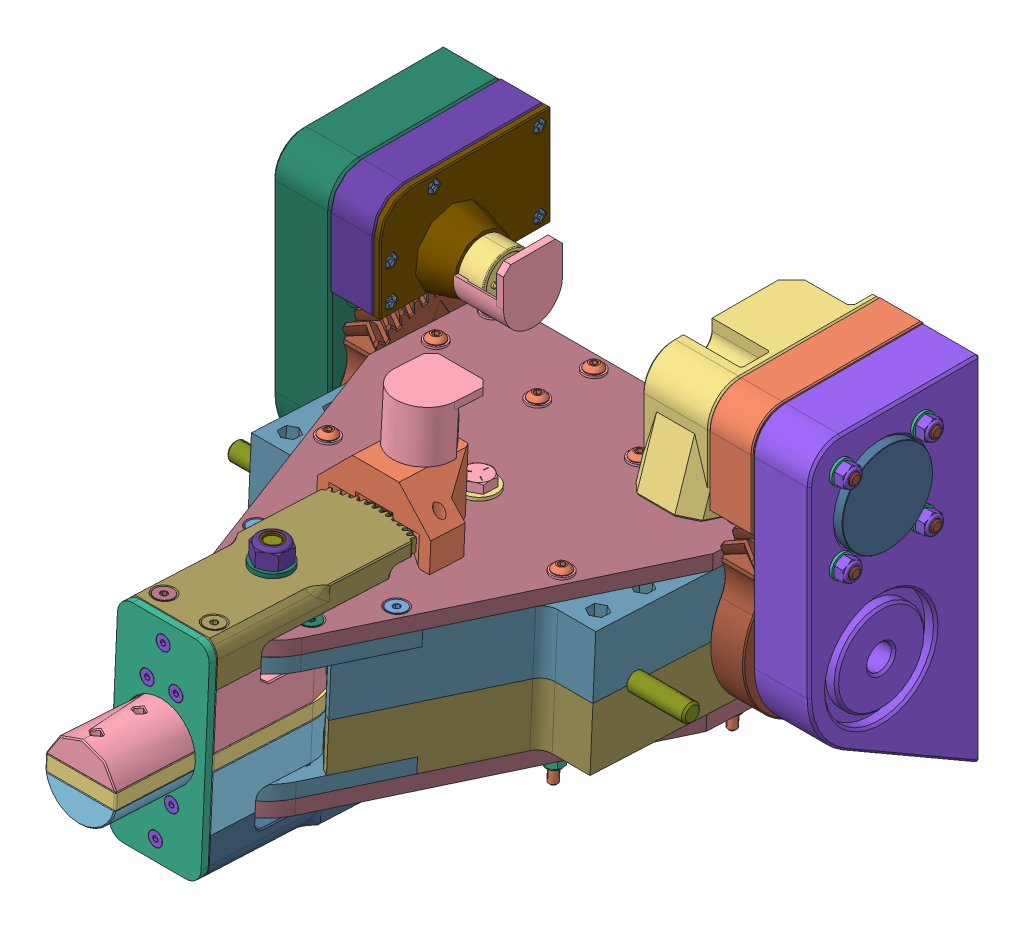
SolidWorks assembly Stick Gimbal Assembly, configuration Default. Lengths in mm. (continued)
Components (placement in the parent): (continued)
- Stick Roll Axis Box Assembly-1: Stick Roll Axis Box Assembly [Default] at (0 0 43.8404) x (1 0 0) z (0 0.047106 0.99889) size (220 126.88 270.74) (continued)
  - 93625A150-7: 93625A150 [Default] at (-22.5 -34.2375 -12.5) x (1 0 0) z (0 -1 0) size (7 8.08 5) (continued)
    - 93625A150-1: 93625A150 [Default] at origin size (6.53 6.53 0.53)
  - 93625A150-8: 93625A150 [Default] at (-22.5 -34.2375 12.5) x (1 0 0) z (0 -1 0) size (7 8.08 5)
    - 93625A150_2-1: 93625A150_2 [Default] at origin size (7 8.08 5)
    - 93625A150-1: 93625A150 [Default] at origin size (6.53 6.53 0.53)
  - 93625A150-9: 93625A150 [Default] at (-51.7 -34.2375 76.04) x (1 0 0) z (0 -1 0) size (7 8.08 5)
    - 93625A150_2-1: 93625A150_2 [Default] at origin size (7 8.08 5)
    - 93625A150-1: 93625A150 [Default] at origin size (6.53 6.53 0.53)
  - 93625A150-10: 93625A150 [Default] at (51.7 -34.2375 76.04) x (1 0 0) z (0 -1 0) size (7 8.08 5)
    - 93625A150_2-1: 93625A150_2 [Default] at origin size (7 8.08 5)
    - 93625A150-1: 93625A150 [Default] at origin size (6.53 6.53 0.53)
  - 92141A029 - 1_4 0.281_ ID, 0.625_ OD Steel Flat Washer-1: 92141A029 - 1_4 0.281_ ID, 0.625_ OD Steel Flat Washer [Default] at (0 -33.3375 61.352) x (1 0 0) z (0 -1 0) size (15.88 15.88 1.45)
  - 92141A029 - 1_4 0.281_ ID, 0.625_ OD Steel Flat Washer-2: 92141A029 - 1_4 0.281_ ID, 0.625_ OD Steel Flat Washer [Default] at (0 33.3375 61.352) x (1 0 0) z (0 1 0) size (15.88 15.88 1.45)
  - 91247A555-1: 91247A555 [Default] at (0 34.7853 61.352) x (1 0 0) z (0 1 0) size (11.11 12.83 86.52)
  - 95615A120-1: 95615A120 [Default] at (0 -34.7853 61.352) x (1 0 0) z (0 -1 0) size (11.11 12.83 7.94)
    - 95615A120-1: 95615A120 [Default] at origin size (11.11 12.83 7.94)
    - 95615A120_2-1: 95615A120_2 [Default] at origin size (10.65 10.65 1.02)
- 93475A280-1: 93475A280 [Default] at (91.2 0 43.8404) x (0 -0.001745 0.999998) z (1 0 0) size (20 20 2.2)
- 93475A280-2: 93475A280 [Default] at (-91.2 0 43.8404) x (0 0.001745 -0.999998) z (-1 0 0) size (20 20 2.2)
- Pitch Bearing Block Asmbly Left-1: Pitch Bearing Block Asmbly Left [Default] at origin size (48 156.22 75.59)
  - Pitch Bearing Block Left-1: Pitch Bearing Block Left [Default] at origin size (25.4 156.22 75.59)
  - 10x30x9mm Sealed Radial Ball Bearing-1: 10x30x9mm Sealed Radial Ball Bearing [Default] at (97.9 0 43.8404) x (0 0 1) z (-1 0 0) size (30 30 9)
  - 93625A200 - M5 x 0.8 mm Nylon-Insert Locknut-1: 93625A200 - M5 x 0.8 mm Nylon-Insert Locknut [Default] at (106.6 76.2 6.35) x (0 1 0) z (0 0 1) size (8 9.24 5)
    - 93625A200 - M5 x 0.8 mm Nylon-Insert Locknut_2-1: 93625A200 - M5 x 0.8 mm Nylon-Insert Locknut_2 [Default] at origin size (8 9.24 5)
    - 93625A200 - M5 x 0.8 mm Nylon-Insert Locknut-1: 93625A200 - M5 x 0.8 mm Nylon-Insert Locknut [Default] at origin size (7.53 7.53 0.53)
  - 93625A200 - M5 x 0.8 mm Nylon-Insert Locknut-2: 93625A200 - M5 x 0.8 mm Nylon-Insert Locknut [Default] at (106.6 19.05 6.35) x (0 -1 0) z (0 0 1) size (8 9.24 5)
    - 93625A200 - M5 x 0.8 mm Nylon-Insert Locknut_2-1: 93625A200 - M5 x 0.8 mm Nylon-Insert Locknut_2 [Default] at origin size (8 9.24 5)
    - 93625A200 - M5 x 0.8 mm Nylon-Insert Locknut-1: 93625A200 - M5 x 0.8 mm Nylon-Insert Locknut [Default] at origin size (7.53 7.53 0.53)
  - 93625A200 - M5 x 0.8 mm Nylon-Insert Locknut-3: 93625A200 - M5 x 0.8 mm Nylon-Insert Locknut [Default] at (106.6 -38.1 6.35) x (0 -1 0) z (0 0 1) size (8 9.24 5)
    - 93625A200 - M5 x 0.8 mm Nylon-Insert Locknut_2-1: 93625A200 - M5 x 0.8 mm Nylon-Insert Locknut_2 [Default] at origin size (8 9.24 5)
    - 93625A200 - M5 x 0.8 mm Nylon-Insert Locknut-1: 93625A200 - M5 x 0.8 mm Nylon-Insert Locknut [Default] at origin size (7.53 7.53 0.53)
  - ACE_FRT-K2-XXX-1: ACE_FRT-K2-XXX [Default] at (121.7 63 43.8404) x (0 -1 0) z (0 0 1) size (47 42 47)
  - 93475A240-1: 93475A240 [Default] at (118.8 45 61.8404) x (0 0 -1) z (1 0 0) size (10 10 1.1)
  - 93475A240-2: 93475A240 [Default] at (118.8 81 61.8404) x (0 0 -1) z (1 0 0) size (10 10 1.1)
  - 93475A240-3: 93475A240 [Default] at (118.8 45 25.8404) x (0 0 -1) z (1 0 0) size (10 10 1.1)
  - 93475A240-4: 93475A240 [Default] at (118.8 81 25.8404) x (0 0 -1) z (1 0 0) size (10 10 1.1)
  - 93625A200 - M5 x 0.8 mm Nylon-Insert Locknut-4: 93625A200 - M5 x 0.8 mm Nylon-Insert Locknut [Default] at (119.9 45 61.8404) x (0 0 1) z (1 0 0) size (8 9.24 5)
    - 93625A200 - M5 x 0.8 mm Nylon-Insert Locknut_2-1: 93625A200 - M5 x 0.8 mm Nylon-Insert Locknut_2 [Default] at origin size (8 9.24 5)
    - 93625A200 - M5 x 0.8 mm Nylon-Insert Locknut-1: 93625A200 - M5 x 0.8 mm Nylon-Insert Locknut [Default] at origin size (7.53 7.53 0.53)
  - 93625A200 - M5 x 0.8 mm Nylon-Insert Locknut-5: 93625A200 - M5 x 0.8 mm Nylon-Insert Locknut [Default] at (119.9 81 61.8404) x (0 0 1) z (1 0 0) size (8 9.24 5)
    - 93625A200 - M5 x 0.8 mm Nylon-Insert Locknut_2-1: 93625A200 - M5 x 0.8 mm Nylon-Insert Locknut_2 [Default] at origin size (8 9.24 5)
    - 93625A200 - M5 x 0.8 mm Nylon-Insert Locknut-1: 93625A200 - M5 x 0.8 mm Nylon-Insert Locknut [Default] at origin size (7.53 7.53 0.53)
  - 93625A200 - M5 x 0.8 mm Nylon-Insert Locknut-6: 93625A200 - M5 x 0.8 mm Nylon-Insert Locknut [Default] at (119.9 81 25.8404) x (0 0 1) z (1 0 0) size (8 9.24 5)
    - 93625A200 - M5 x 0.8 mm Nylon-Insert Locknut_2-1: 93625A200 - M5 x 0.8 mm Nylon-Insert Locknut_2 [Default] at origin size (8 9.24 5)
    - 93625A200 - M5 x 0.8 mm Nylon-Insert Locknut-1: 93625A200 - M5 x 0.8 mm Nylon-Insert Locknut [Default] at origin size (7.53 7.53 0.53)
  - 93625A200 - M5 x 0.8 mm Nylon-Insert Locknut-7: 93625A200 - M5 x 0.8 mm Nylon-Insert Locknut [Default] at (119.9 45 25.8404) x (0 0 1) z (1 0 0) size (8 9.24 5)
    - 93625A200 - M5 x 0.8 mm Nylon-Insert Locknut_2-1: 93625A200 - M5 x 0.8 mm Nylon-Insert Locknut_2 [Default] at origin size (8 9.24 5)
    - 93625A200 - M5 x 0.8 mm Nylon-Insert Locknut-1: 93625A200 - M5 x 0.8 mm Nylon-Insert Locknut [Default] at origin size (7.53 7.53 0.53)
  - 91292A129-1: 91292A129 [Default] at (100.7 45 61.8404) x (0 0 -1) z (-1 0 0) size (8.5 8.5 30.23)
  - 91292A129-2: 91292A129 [Default] at (100.7 81 25.8404) x (0 0 -1) z (-1 0 0) size (8.5 8.5 30.23)
  - 91292A129-3: 91292A129 [Default] at (100.7 81 61.8404) x (0 0 -1) z (-1 0 0) size (8.5 8.5 30.23)
  - 91292A129-4: 91292A129 [Default] at (100.7 45 25.8404) x (0 0 -1) z (-1 0 0) size (8.5 8.5 30.23)
  - Pitch Damper Gear Small Asmbly Left-1: Pitch Damper Gear Small Asmbly Left [Default] at origin size (12 40.1 40.09)
    - Pitch Damper Gear Small Left-1: Pitch Damper Gear Small Left [Default] at (83.7 63 43.8404) x (0 0 -1) z (-1 0 0) size (40.09 40.1 12)
    - 91828A231 - M4 x 0.7mm Hex Nut-1: 91828A231 - M4 x 0.7mm Hex Nut [Default] at (83.7 71.4 43.8404) x (0 0 -1) z (0 1 0) size (7 8.08 3.2)
    - 91390A114-1: 91390A114 [Default] at (83.7 75.0173 43.8404) x (0 0 -1) z (0 1 0) size (3.91 3.91 10.12)
  - 94180A331-1: 94180A331 [Default] at (93.4 55.0625 70.5904) x (0 0 1) z (-1 0 0) size (5.56 5.56 3.8)
  - 94180A331-2: 94180A331 [Default] at (93.4 70.9375 70.5904) x (0 0 1) z (-1 0 0) size (5.56 5.56 3.8)
  - 94180A331-3: 94180A331 [Default] at (93.4 89.75 51.7779) x (0 0 1) z (-1 0 0) size (5.56 5.56 3.8)
  - 94180A331-4: 94180A331 [Default] at (93.4 89.75 5) x (0 0 1) z (-1 0 0) size (5.56 5.56 3.8)
  - 94180A331-5: 94180A331 [Default] at (93.4 55.0625 5) x (0 0 1) z (-1 0 0) size (5.56 5.56 3.8)
- Pitch Bearing Block Asmbly Right-1: Pitch Bearing Block Asmbly Right [Default] x (-1 0 0) z (0 0 -1) size (55.53 156.22 75.59)
  - Pitch Bearing Block Right-1: Pitch Bearing Block Right [Default] at origin size (25.4 156.22 75.59)
  - 10x30x9mm Sealed Radial Ball Bearing-1: 10x30x9mm Sealed Radial Ball Bearing [Default] at (97.9 0 -43.8404) x (0 0 -1) z (1 0 0) size (30 30 9)
  - ACE_FRT-K2-XXX-1: ACE_FRT-K2-XXX [Default] at (121.7 63 -43.8404) x (0 -1 0) z (0 0 1) size (47 42 47)
  - 93475A240-1: 93475A240 [Default] at (118.8 81 -61.8404) x (0 0 1) z (1 0 0) size (10 10 1.1)
  - 93475A240-2: 93475A240 [Default] at (118.8 45 -25.8404) x (0 0 1) z (1 0 0) size (10 10 1.1)
  - 93475A240-3: 93475A240 [Default] at (118.8 81 -25.8404) x (0 0 1) z (1 0 0) size (10 10 1.1)
  - 93475A240-4: 93475A240 [Default] at (118.8 45 -61.8404) x (0 0 1) z (1 0 0) size (10 10 1.1)
  - 93625A200 - M5 x 0.8 mm Nylon-Insert Locknut-1: 93625A200 - M5 x 0.8 mm Nylon-Insert Locknut [Default] at (119.9 81 -61.8404) x (0 0 1) z (1 0 0) size (8 9.24 5)
    - 93625A200 - M5 x 0.8 mm Nylon-Insert Locknut_2-1: 93625A200 - M5 x 0.8 mm Nylon-Insert Locknut_2 [Default] at origin size (8 9.24 5)
    - 93625A200 - M5 x 0.8 mm Nylon-Insert Locknut-1: 93625A200 - M5 x 0.8 mm Nylon-Insert Locknut [Default] at origin size (7.53 7.53 0.53)
  - 93625A200 - M5 x 0.8 mm Nylon-Insert Locknut-2: 93625A200 - M5 x 0.8 mm Nylon-Insert Locknut [Default] at (119.9 45 -61.8404) x (0 0 1) z (1 0 0) size (8 9.24 5)
    - 93625A200 - M5 x 0.8 mm Nylon-Insert Locknut_2-1: 93625A200 - M5 x 0.8 mm Nylon-Insert Locknut_2 [Default] at origin size (8 9.24 5)
    - 93625A200 - M5 x 0.8 mm Nylon-Insert Locknut-1: 93625A200 - M5 x 0.8 mm Nylon-Insert Locknut [Default] at origin size (7.53 7.53 0.53)
  - 93625A200 - M5 x 0.8 mm Nylon-Insert Locknut-3: 93625A200 - M5 x 0.8 mm Nylon-Insert Locknut [Default] at (119.9 81 -25.8404) x (0 0 1) z (1 0 0) size (8 9.24 5)
    - 93625A200 - M5 x 0.8 mm Nylon-Insert Locknut_2-1: 93625A200 - M5 x 0.8 mm Nylon-Insert Locknut_2 [Default] at origin size (8 9.24 5)
    - 93625A200 - M5 x 0.8 mm Nylon-Insert Locknut-1: 93625A200 - M5 x 0.8 mm Nylon-Insert Locknut [Default] at origin size (7.53 7.53 0.53)
  - 93625A200 - M5 x 0.8 mm Nylon-Insert Locknut-4: 93625A200 - M5 x 0.8 mm Nylon-Insert Locknut [Default] at (119.9 45 -25.8404) x (0 0 1) z (1 0 0) size (8 9.24 5)
    - 93625A200 - M5 x 0.8 mm Nylon-Insert Locknut_2-1: 93625A200 - M5 x 0.8 mm Nylon-Insert Locknut_2 [Default] at origin size (8 9.24 5)
    - 93625A200 - M5 x 0.8 mm Nylon-Insert Locknut-1: 93625A200 - M5 x 0.8 mm Nylon-Insert Locknut [Default] at origin size (7.53 7.53 0.53)
  - 91292A129-1: 91292A129 [Default] at (100.7 81 -61.8404) x (0 0 1) z (-1 0 0) size (8.5 8.5 30.23)
  - 91292A129-2: 91292A129 [Default] at (100.7 45 -61.8404) x (0 0 1) z (-1 0 0) size (8.5 8.5 30.23)
  - 91292A129-3: 91292A129 [Default] at (100.7 45 -25.8404) x (0 0 1) z (-1 0 0) size (8.5 8.5 30.23)
  - 91292A129-4: 91292A129 [Default] at (100.7 81 -25.8404) x (0 0 1) z (-1 0 0) size (8.5 8.5 30.23)
  - 93625A200 - M5 x 0.8 mm Nylon-Insert Locknut-5: 93625A200 - M5 x 0.8 mm Nylon-Insert Locknut [Default] at (106.6 -38.1 -6.35) x (0 1 0) z (0 0 -1) size (8 9.24 5)
    - 93625A200 - M5 x 0.8 mm Nylon-Insert Locknut_2-1: 93625A200 - M5 x 0.8 mm Nylon-Insert Locknut_2 [Default] at origin size (8 9.24 5)
    - 93625A200 - M5 x 0.8 mm Nylon-Insert Locknut-1: 93625A200 - M5 x 0.8 mm Nylon-Insert Locknut [Default] at origin size (7.53 7.53 0.53)
  - 93625A200 - M5 x 0.8 mm Nylon-Insert Locknut-6: 93625A200 - M5 x 0.8 mm Nylon-Insert Locknut [Default] at (106.6 19.05 -6.35) x (0 1 0) z (0 0 -1) size (8 9.24 5)
    - 93625A200 - M5 x 0.8 mm Nylon-Insert Locknut_2-1: 93625A200 - M5 x 0.8 mm Nylon-Insert Locknut_2 [Default] at origin size (8 9.24 5)
    - 93625A200 - M5 x 0.8 mm Nylon-Insert Locknut-1: 93625A200 - M5 x 0.8 mm Nylon-Insert Locknut [Default] at origin size (7.53 7.53 0.53)
  - 93625A200 - M5 x 0.8 mm Nylon-Insert Locknut-7: 93625A200 - M5 x 0.8 mm Nylon-Insert Locknut [Default] at (106.6 76.2 -6.35) x (0 1 0) z (0 0 -1) size (8 9.24 5)
    - 93625A200 - M5 x 0.8 mm Nylon-Insert Locknut_2-1: 93625A200 - M5 x 0.8 mm Nylon-Insert Locknut_2 [Default] at origin size (8 9.24 5)
    - 93625A200 - M5 x 0.8 mm Nylon-Insert Locknut-1: 93625A200 - M5 x 0.8 mm Nylon-Insert Locknut [Default] at origin size (7.53 7.53 0.53)
  - Pitch Damper Gear Small Asmbly Right-1: Pitch Damper Gear Small Asmbly Right [Default] x (-1 0 0) z (0 0 -1) size (19.53 40.1 40.09)
    - Pitch Damper Gear Small Left_1-1: Pitch Damper Gear Small Left_1 [Default] at (-83.7 63 43.8404) x (0 0 1) z (1 0 0) size (40.09 40.1 19.53)
    - 91828A231 - M4 x 0.7mm Hex Nut-1: 91828A231 - M4 x 0.7mm Hex Nut [Default] at (-83.7 71.4 43.8404) x (0 0 1) z (0 1 0) size (7 8.08 3.2)
    - 91390A114-1: 91390A114 [Default] at (-83.7 75.0173 43.8404) x (0 0 1) z (0 1 0) size (3.91 3.91 10.12)
  - 94180A331-1: 94180A331 [Default] at (93.4 55.0625 -70.5904) x (0 0 -1) z (-1 0 0) size (5.56 5.56 3.8)
  - 94180A331-2: 94180A331 [Default] at (93.4 70.9375 -70.5904) x (0 0 -1) z (-1 0 0) size (5.56 5.56 3.8)
  - 94180A331-3: 94180A331 [Default] at (93.4 89.75 -51.7779) x (0 0 -1) z (-1 0 0) size (5.56 5.56 3.8)
  - 94180A331-4: 94180A331 [Default] at (93.4 89.75 -5) x (0 0 -1) z (-1 0 0) size (5.56 5.56 3.8)
  - 94180A331-5: 94180A331 [Default] at (93.4 55.0625 -5) x (0 0 -1) z (-1 0 0) size (5.56 5.56 3.8)
- Pitch Sensor Assembly Left(Mirror)-1: Pitch Sensor Assembly Left(Mirror) [Default] x (-1 0 0) z (0 0 -1) size (49.36 44.45 75.59)
  - Pitch Sensor Assembly Left(Mirror)-1: Pitch Sensor Assembly Left(Mirror) [Default] at origin size (19.05 44.45 75.59)
  - Pitch Sensor Assembly Left(Mirror)_2-1: Pitch Sensor Assembly Left(Mirror)_2 [Default] at origin size (16.83 44.45 75.59)
  - 6127V1AxxxL.5FS-1: 6127V1AxxxL.5FS [6127V1A90L.5FS] at (57.3734 63 -43.8404) x (0 -1 0) z (0 0 -1) size (22.23 35.66 22.23)
- 91420A130 - FHS, 90 DEG, M3-0.5 X 25, STEEL, ZINC-1: 91420A130 - FHS, 90 DEG, M3-0.5 X 25, STEEL, ZINC [91420A130] at (-73.1746 55.0625 70.5904) x (0 -0.432202 -0.901777) z (1 0 0) size (5.6 5.6 25.28)
- 91420A130 - FHS, 90 DEG, M3-0.5 X 25, STEEL, ZINC-2: 91420A130 - FHS, 90 DEG, M3-0.5 X 25, STEEL, ZINC [91420A130] at (-73.1746 70.9375 70.5904) x (0 -0.283756 -0.958897) z (1 0 0) size (5.6 5.6 25.28)
- 91420A130 - FHS, 90 DEG, M3-0.5 X 25, STEEL, ZINC-4: 91420A130 - FHS, 90 DEG, M3-0.5 X 25, STEEL, ZINC [91420A130] at (-73.1746 89.75 51.7779) x (0 -0.159348 -0.987223) z (1 0 0) size (5.6 5.6 25.28)
- 91420A130 - FHS, 90 DEG, M3-0.5 X 25, STEEL, ZINC-6: 91420A130 - FHS, 90 DEG, M3-0.5 X 25, STEEL, ZINC [91420A130] at (-73.1746 89.75 5) x (0 -0.066633 -0.997778) z (1 0 0) size (5.6 5.6 25.28)
- 91420A130 - FHS, 90 DEG, M3-0.5 X 25, STEEL, ZINC-8: 91420A130 - FHS, 90 DEG, M3-0.5 X 25, STEEL, ZINC [91420A130] at (-73.1746 55.0625 5) x (0 -0.012216 -0.999925) z (1 0 0) size (5.6 5.6 25.28)
- Left Damper Debris Shield-2: Left Damper Debris Shield [Default] at origin size (48.58 60.12 84.36)
  - Left Damper Debris Shield Spacer-1: Left Damper Debris Shield Spacer [Default] at origin size (19.05 44.45 75.59)
  - Left Damper Debris Shield Top Plate-1: Left Damper Debris Shield Top Plate [Default] at origin size (29.53 60.12 84.36)
- 91420A130 - FHS, 90 DEG, M3-0.5 X 25, STEEL, ZINC-14: 91420A130 - FHS, 90 DEG, M3-0.5 X 25, STEEL, ZINC [91420A130] at (73.1746 55.0625 70.5904) x (0 0.432202 0.901777) z (-1 0 0) size (5.6 5.6 25.28)
- 91420A130 - FHS, 90 DEG, M3-0.5 X 25, STEEL, ZINC-15: 91420A130 - FHS, 90 DEG, M3-0.5 X 25, STEEL, ZINC [91420A130] at (73.1746 70.9375 70.5904) x (0 0.283756 0.958897) z (-1 0 0) size (5.6 5.6 25.28)
- 91420A130 - FHS, 90 DEG, M3-0.5 X 25, STEEL, ZINC-16: 91420A130 - FHS, 90 DEG, M3-0.5 X 25, STEEL, ZINC [91420A130] at (73.1746 89.75 51.7779) x (0 0.159348 0.987223) z (-1 0 0) size (5.6 5.6 25.28)
- 91420A130 - FHS, 90 DEG, M3-0.5 X 25, STEEL, ZINC-17: 91420A130 - FHS, 90 DEG, M3-0.5 X 25, STEEL, ZINC [91420A130] at (73.1746 89.75 5) x (0 0.066633 0.997778) z (-1 0 0) size (5.6 5.6 25.28)
- 91420A130 - FHS, 90 DEG, M3-0.5 X 25, STEEL, ZINC-18: 91420A130 - FHS, 90 DEG, M3-0.5 X 25, STEEL, ZINC [91420A130] at (73.1746 55.0625 5) x (0 0.012216 0.999925) z (-1 0 0) size (5.6 5.6 25.28)
- Hall Sensor Cable Cover-1: Hall Sensor Cable Cover [Default] at (0 64.9361 128.2075) x (1 0 0) z (0 0.998254 -0.059067) size (26.04 28.89 22.23)
- Hall Sensor Cable Cover-2: Hall Sensor Cable Cover [Default] at (-57.5225 63 43.8404) x (0 0 -1) z (1 0 0) size (26.04 28.89 22.23)
Mates (geometry in assembly coordinates):
- Concentric1: concentric anti-aligned: cylinder of Stick Roll Axis Box Assembly-1/Main Casing Asmbly-1/Pitch Axis Rod-1 through (0 0 43.8404) axis (1 0 0) radius 5; cylinder of Pitch Bearing Block Asmbly Left-1/10x30x9mm Sealed Radial Ball Bearing-1 through (97.9 0 43.8404) axis (-1 0 0) radius 5
- Width1: width anti-aligned: plane of Stick Roll Axis Box Assembly-1/Main Casing Asmbly-1/Pitch Axis Rod-1 through (-110 0 43.8404) normal (-1 0 0); plane of 93475A280-2 through (110 0 43.8404) normal (1 0 0); plane of Stick Roll Axis Box Assembly-1/Main Casing Asmbly-1/Pitch Axis Rod-1 through (-91.2 0 43.8404) normal (1 0 0); plane of 93475A280-1 through (91.2 0 43.8404) normal (-1 0 0)
- Pitch Neutral Position: planar angle = 0.047124 rad aligned: plane of Stick Roll Axis Box Assembly-1/Aft Plate Assembly-1/Main Plate Sub Asmbly_1-1/Main Plate-1 through (0 37.0488 121.7528) normal (0 0.99889 -0.047106); plane of Pitch Bearing Block Asmbly Left-1/Pitch Bearing Block Left-1 through (93.4 94.75 0) normal (0 1 0)
- LimitAngle3: limit planar angle = 0.270526 rad aligned: plane of Stick Roll Axis Box Assembly-1/Aft Plate Assembly-1/Main Plate Sub Asmbly_1-1/Main Plate-1 through (0 37.0488 121.7528) normal (0 0.99889 -0.047106); plane of Pitch Bearing Block Asmbly Left-1/Pitch Bearing Block Left-1 through (93.4 94.75 0) normal (0 1 0)
- Concentric3: concentric: cylinder of Pitch Bearing Block Asmbly Right-1/Pitch Damper Gear Small Asmbly Right-1/Pitch Damper Gear Small Left_1-1 through (-77.7 63 43.8404) axis (1 0 0) radius 3; cylinder of Pitch Sensor Assembly Left(Mirror)-1/6127V1AxxxL.5FS-1 through (-81.0475 63 43.8404) axis (1 0 0) radius 3.1712
- Parallel2: parallel: plane of Pitch Bearing Block Asmbly Right-1/Pitch Damper Gear Small Asmbly Right-1/Pitch Damper Gear Small Left_1-1 through (-77.7 69.6 47.3404) normal (0 1 0); plane of Pitch Sensor Assembly Left(Mirror)-1/6127V1AxxxL.5FS-1 through (-69.7 65.3152 46.0075) normal (0 1 0)
- Coincident2: coincident: plane of Pitch Bearing Block Asmbly Right-1/ACE_FRT-K2-XXX-1 through (-79.7 61.6 43.8404) normal (1 0 0); plane of Pitch Sensor Assembly Left(Mirror)-1/6127V1AxxxL.5FS-1 through (-79.7 63 43.8404) normal (-1 0 0)
- Concentric36: concentric anti-aligned: cylinder of Stick Roll Axis Box Assembly-1/Aft Plate Assembly-1/Roll Sensor Asmbly-1/6127V1AxxxL.5FS-1 through (0 64.7188 128.2204) axis (0 0.998254 -0.059067) radius 11.1125; cylinder of Hall Sensor Cable Cover-1 through (0 83.9529 127.0823) axis (0 -0.998254 0.059067) radius 13.0175
- Coincident44: coincident: plane of Stick Roll Axis Box Assembly-1/Aft Plate Assembly-1/Roll Sensor Asmbly-1/Roll Sensor Mount Main-1 through (-20 65.4735 140.1775) normal (0 0.99889 -0.047106); point of Hall Sensor Cable Cover-1
- Concentric37: concentric anti-aligned: cylinder of Pitch Sensor Assembly Left(Mirror)-1/6127V1AxxxL.5FS-1 through (-57.9436 63 43.8404) axis (1 0 0) radius 11.1125; cylinder of Hall Sensor Cable Cover-2 through (-38.4725 63 43.8404) axis (-1 0 0) radius 13.0175
- Coincident45: coincident: plane of Pitch Sensor Assembly Left(Mirror)-1/Pitch Sensor Assembly Left(Mirror)_2-1 through (-57.5225 63 43.8404) normal (1 0 0); point of Hall Sensor Cable Cover-2
- Concentric38: concentric aligned: cone of Pitch Sensor Assembly Left(Mirror)-1/Pitch Sensor Assembly Left(Mirror)_2-1 through (-71.175 55.0625 70.5904) axis (-1 0 0); cone of 91420A130 - FHS, 90 DEG, M3-0.5 X 25, STEEL, ZINC-1 through (-71.5246 55.0625 70.5904) axis (-1 0 0)
- Coincident46: coincident aligned: cone of Pitch Sensor Assembly Left(Mirror)-1/Pitch Sensor Assembly Left(Mirror)_2-1 through (-71.175 55.0625 70.5904) axis (-1 0 0); cone of 91420A130 - FHS, 90 DEG, M3-0.5 X 25, STEEL, ZINC-1 through (-71.5246 55.0625 70.5904) axis (-1 0 0)
- Concentric39: concentric aligned: cone of Pitch Sensor Assembly Left(Mirror)-1/Pitch Sensor Assembly Left(Mirror)_2-1 through (-71.175 70.9375 70.5904) axis (-1 0 0); cone of 91420A130 - FHS, 90 DEG, M3-0.5 X 25, STEEL, ZINC-2 through (-71.5246 70.9375 70.5904) axis (-1 0 0)
- Coincident47: coincident aligned: cone of Pitch Sensor Assembly Left(Mirror)-1/Pitch Sensor Assembly Left(Mirror)_2-1 through (-71.175 70.9375 70.5904) axis (-1 0 0); cone of 91420A130 - FHS, 90 DEG, M3-0.5 X 25, STEEL, ZINC-2 through (-71.5246 70.9375 70.5904) axis (-1 0 0)
- Concentric40: concentric aligned: cone of Pitch Sensor Assembly Left(Mirror)-1/Pitch Sensor Assembly Left(Mirror)_2-1 through (-71.175 89.75 51.7779) axis (-1 0 0); cone of 91420A130 - FHS, 90 DEG, M3-0.5 X 25, STEEL, ZINC-4 through (-71.5246 89.75 51.7779) axis (-1 0 0)
- Coincident48: coincident aligned: cone of Pitch Sensor Assembly Left(Mirror)-1/Pitch Sensor Assembly Left(Mirror)_2-1 through (-71.175 89.75 51.7779) axis (-1 0 0); cone of 91420A130 - FHS, 90 DEG, M3-0.5 X 25, STEEL, ZINC-4 through (-71.5246 89.75 51.7779) axis (-1 0 0)
- Concentric41: concentric aligned: cone of Pitch Sensor Assembly Left(Mirror)-1/Pitch Sensor Assembly Left(Mirror)_2-1 through (-71.175 89.75 5) axis (-1 0 0); cone of 91420A130 - FHS, 90 DEG, M3-0.5 X 25, STEEL, ZINC-6 through (-71.5246 89.75 5) axis (-1 0 0)
- Coincident49: coincident aligned: cone of Pitch Sensor Assembly Left(Mirror)-1/Pitch Sensor Assembly Left(Mirror)_2-1 through (-71.175 89.75 5) axis (-1 0 0); cone of 91420A130 - FHS, 90 DEG, M3-0.5 X 25, STEEL, ZINC-6 through (-71.5246 89.75 5) axis (-1 0 0)
- Concentric42: concentric aligned: cone of Pitch Sensor Assembly Left(Mirror)-1/Pitch Sensor Assembly Left(Mirror)_2-1 through (-71.175 55.0625 5) axis (-1 0 0); cone of 91420A130 - FHS, 90 DEG, M3-0.5 X 25, STEEL, ZINC-8 through (-71.5246 55.0625 5) axis (-1 0 0)
- Coincident50: coincident aligned: cone of Pitch Sensor Assembly Left(Mirror)-1/Pitch Sensor Assembly Left(Mirror)_2-1 through (-71.175 55.0625 5) axis (-1 0 0); cone of 91420A130 - FHS, 90 DEG, M3-0.5 X 25, STEEL, ZINC-8 through (-71.5246 55.0625 5) axis (-1 0 0)
- Parallel3: parallel aligned: plane of Pitch Sensor Assembly Left(Mirror)-1/Pitch Sensor Assembly Left(Mirror)-1 through (-74.35 81 75.5904) normal (0 0 1); plane of Hall Sensor Cable Cover-2 through (-68.9657 63 56.8579) normal (0 0 1)
- Parallel7: parallel: line of Stick Roll Axis Box Assembly-1/Aft Plate Assembly-1/Roll Sensor Asmbly-1/Roll Sensor Mount Main-1 through (-25.08 50.4019 134.293) axis (0 0.047106 0.99889); plane of Hall Sensor Cable Cover-1 through (-13.0175 53.5129 128.8834) normal (-1 0 0)
